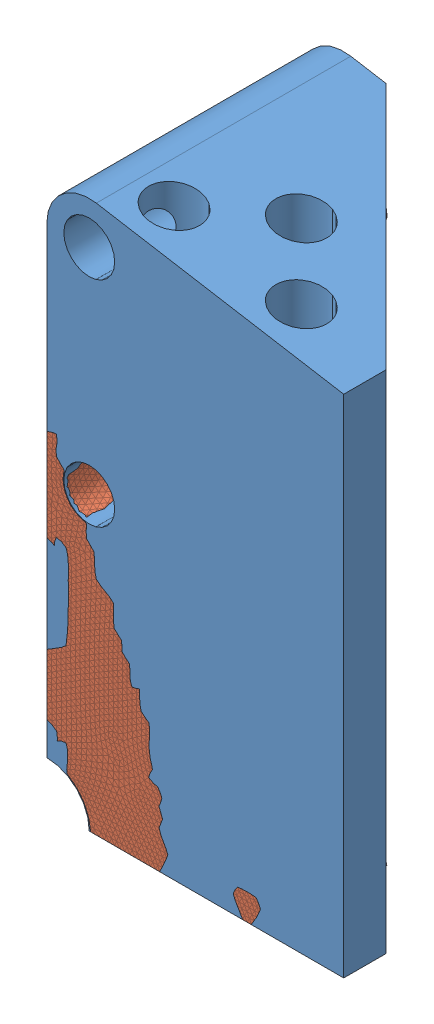
SolidWorks assembly suporte_freio_traseiro_v2_topopt, configuration Default. Lengths in mm.
Overall size (70 129.21 60).
2 component instances, 2 part files, 3 mates.
Components (placement in the parent):
- suporte_freio_traseiro_v2-1: suporte_freio_traseiro_v2 [Default] at (19.4755 7.2205 68.1708) size (70 129.21 60)
- suporte_freio_traseiro_v2_topopt_mesh-1: suporte_freio_traseiro_v2_topopt_mesh [Default] at (19.4811 7.2288 68.1708) size (62.77 125.1 60)
Mates (geometry in assembly coordinates):
- Concentric1: concentric anti-aligned: circle of suporte_freio_traseiro_v2-1; circle of suporte_freio_traseiro_v2_topopt_mesh-1
- Parallel1: parallel: plane of suporte_freio_traseiro_v2-1 through (9.4755 137.2205 128.1708) normal (-1 0 0); line of suporte_freio_traseiro_v2_topopt_mesh-1 through (9.4811 26.4497 127.054) axis (0 0.423737 -0.905785)
- Coincident2: coincident: plane of suporte_freio_traseiro_v2-1 through (19.4755 7.2205 128.1708) normal (0 0 1); line of suporte_freio_traseiro_v2_topopt_mesh-1 through (10.6398 26.6079 128.1708) axis (0.001501 -0.999999 0)
